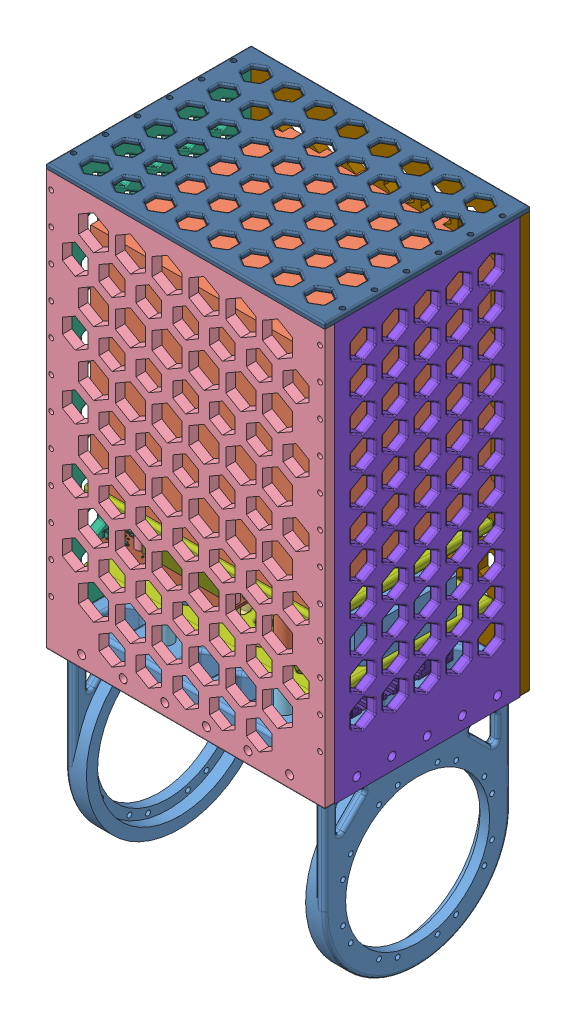
SolidWorks assembly upperbody, configuration 默认. Lengths in mm.
Overall size (174 383 128).
497 component instances, 113 part files, 71 mates.
Components (placement in the parent):
- crotch-1: crotch [默认] at (4.5084 -17.0112 162) size (162 138.05 116)
- battery-1: battery [默认] at (3.2915 206.5588 214.1011) x (-1 0 0) z (0 -1 0) size (140 115 140)
- imu-1: imu [默认] at (5.7743 27.9888 133.0371) x (0 0 -1) z (0 1 0) size (79.76 40 69.46)
- front-1: front [默认] at (4.5084 194.9888 220) size (174 260 6)
- M8螺柱-1: M8螺柱 [默认] at (42.5084 62.9888 122) size (10 25 10)
- M8螺柱-2: M8螺柱 [默认] at (42.5084 62.9888 202) x (0.721666 0 -0.692241) z (0.692241 0 0.721666) size (10 25 10)
- M8螺柱-3: M8螺柱 [默认] at (-32.4916 62.9888 122) x (0.928948 0 -0.370211) z (0.370211 0 0.928948) size (10 25 10)
- M8螺柱-4: M8螺柱 [默认] at (-32.4916 62.9888 202) x (0.697956 0 -0.71614) z (0.71614 0 0.697956) size (10 25 10)
- left-1: left [默认] at (-82.4916 204.9888 162) x (0 0 -1) z (1 0 0) size (116 260 6)
- ctrlbox-2: ctrlbox [默认] at (5.0084 87.9888 162) size (148 6 110)
- right-1: right [默认] at (91.5084 204.9888 162) x (0 0 1) z (-1 0 0) size (116 260 6)
- back-2: back [默认] at (4.5084 194.9888 98) size (174 260 6)
- top-1: top [默认] at (4.5084 304.9888 162) size (174 3 128)
- jetsonnano-1: jetsonnano [默认] at (-39.9804 116.3688 223.5192) x (0 0 1) z (0 1 0) size (100.18 80.53 31.78)
  - 675_13541_batuu_dev_kit_top_ass_asm.stp-1: 675_13541_batuu_dev_kit_top_ass_asm.stp [Default] at (-107.5192 -7.5112 -12.38) size (100.18 80.53 31.78)
    - 642-13541_BATUU_SYS_BOM_ASM.stp-1: 642-13541_BATUU_SYS_BOM_ASM.stp [Default] at origin size (100.18 80.53 21.55)
      - 600-13542-BASE-A02_ASM.stp-1: 600-13542-BASE-A02_ASM.stp [Default] at origin size (100.18 80.53 21.55)
        - 600-13542-BASE-A02.stp-1: 600-13542-BASE-A02.stp [Default] at origin size (100 79 1.57)
        - 064-0473-000_1.stp-1: 064-0473-000_1.stp [Default] at (2.055 -14.41 1.57) size (11.16 8.51 5.94)
        - LOGO_SILK_180_I560.stp-1: LOGO_SILK_180_I560.stp [Default] at (2.088 17.507 0) x (0 1 0) z (0 0 -1) size (14.3 1.27 0.05)
        - LOGO_SILK_POSTAL_ADDRESS.stp-1: LOGO_SILK_POSTAL_ADDRESS.stp [Default] at (3.985 7.597 0) x (0 1 0) z (0 0 -1) size (18.11 2.17 0.05)
        - LS_ICES_I0925X0040_CLASS_B.stp-1: LS_ICES_I0925X0040_CLASS_B.stp [Default] at (0.822 15.645 0) x (0 1 0) z (0 0 -1) size (17.94 1.42 0.03)
        - LOGO_SILK_P3542.stp-1: LOGO_SILK_P3542.stp [Default] at (-1.446 36.987 0) x (0 1 0) z (0 0 -1) size (6.18 1.16 0.01)
        - LOGO_SILK_ROHS_I0300X0153.stp-1: LOGO_SILK_ROHS_I0300X0153.stp [Default] at (0.509 33.093 0) x (0 1 0) z (0 0 -1) size (7.55 3.9 0.05)
        - LOGO_SILK_NVIDIA_I0400X0240.stp-1: LOGO_SILK_NVIDIA_I0400X0240.stp [Default] at (10.037 11.31 0) x (0 1 0) z (0 0 -1) size (7.63 5.72 0.1)
        - 115-1921-000_3.stp-1: 115-1921-000_3.stp [Default] at (71 38 1.57) x (0 -1 0) z (0 0 1) size (5 4 1.01)
        - 115-1921-000_3.stp-2: 115-1921-000_3.stp [Default] at (71 46.5 1.57) x (0 -1 0) z (0 0 1) size (5 4 1.01)
        - 115-1921-000_3.stp-3: 115-1921-000_3.stp [Default] at (71 29.5 1.57) x (0 -1 0) z (0 0 1) size (5 4 1.01)
        - LS_CTUVUS_0500X0500_SIMPLE.stp-1: LS_CTUVUS_0500X0500_SIMPLE.stp [Default] at (49.36 31.942 0) x (-1 0 0) z (0 0 -1) size (5.04 5.01 0.05)
        - LOGO_SILK_UKRAINE_0500X0500.stp-1: LOGO_SILK_UKRAINE_0500X0500.stp [Default] at (41 32.494 0) x (-1 0 0) z (0 0 -1) size (4.37 5.01 0.05)
        - LOGO_SILK_SAA_1206X0540.stp-1: LOGO_SILK_SAA_1206X0540.stp [Default] at (44.276 41.966 0) x (-1 0 0) z (0 0 -1) size (12.08 8.03 0.06)
        - 064-0476-000_1.stp-1: 064-0476-000_1.stp [Default] at (55.6 -9.269 1.57) size (14.86 17.99 18.47)
        - 064-0472-000_1.stp-1: 064-0472-000_1.stp [Default] at (88 -14.3 1.57) size (8.8 6.34 3.46)
        - 0402_SHUNT_NO.stp-1: 0402_SHUNT_NO.stp [Default] at (57.444 37.6 1.57) size (1.51 0.51 0.03)
        - 0402_SHUNT_NO.stp-2: 0402_SHUNT_NO.stp [Default] at (55.15 36.025 1.57) x (0 1 0) z (0 0 1) size (1.51 0.51 0.03)
        - 0402_SHUNT_NO.stp-3: 0402_SHUNT_NO.stp [Default] at (55.15 33.762 1.57) x (0 -1 0) z (0 0 1) size (1.51 0.51 0.03)
        - 0402_SHORT.stp-1: 0402_SHORT.stp [Default] at (57.6 38.53 1.57) size (1.51 0.51 1)
        - 0402_SHORT.stp-2: 0402_SHORT.stp [Default] at (53.708 35.675 1.57) x (-1 0 0) z (0 0 1) size (1.51 0.51 1)
        - 0402_SHORT.stp-3: 0402_SHORT.stp [Default] at (53.708 34.112 1.57) x (-1 0 0) z (0 0 1) size (1.51 0.51 1)
        - 0402_SHORT.stp-4: 0402_SHORT.stp [Default] at (60.9 37.1 1.57) x (0 -1 0) z (0 0 1) size (1.51 0.51 1)
        - 064-0474-000_1.stp-1: 064-0474-000_1.stp [Default] at (38.6 -9.759 1.57) size (14.81 17.11 9.91)
        - 085-0347-000_1.stp-1: 085-0347-000_1.stp [Default] at (31.173 31.804 1.57) x (0 -1 0) z (0 0 1) size (3.6 2.9 0.81)
        - 115-2844-000_1.stp-1: 115-2844-000_1.stp [Default] at (39.89 33.254 1.57) x (0 1 0) z (0 0 1) size (5.01 7.06 1.76)
        - 074-0259-000_1.stp-1: 074-0259-000_1.stp [Default] at (19.751 -12.06 1.57) x (0 1 0) z (0 0 1) size (13.02 16.16 8.1)
        - 106-0078-000_1.stp-1: 106-0078-000_1.stp [Default] at (4.864 -6.11 1.57) size (6.08 4.44 1.61)
        - LOGO_SILK_EAC_050X050.stp-1: LOGO_SILK_EAC_050X050.stp [Default] at (28.157 35.506 0) x (-1 0 0) z (0 0 -1) size (5 5 0.05)
        - LOGO_LABEL_PPID_0180X0050.stp-1: LOGO_LABEL_PPID_0180X0050.stp [Default] at (49.45 19.35 0) x (-1 0 0) z (0 0 -1) size (18 5 0.15)
        - 074-0221-000_3.stp-1: 074-0221-000_3.stp [Default] at (86 29 1.57) x (0 1 0) z (0 0 1) size (51.01 5.29 12.01)
        - 080-1656-000_3.stp-1: 080-1656-000_3.stp [Default] at (44 16.6 1.57) x (-1 0 0) z (0 0 1) size (77.5 26.11 9.91)
        - 080-1669-000_2.stp-1: 080-1669-000_2.stp [Default] at (0.2 29 1.57) x (0 -1 0) z (0 0 1) size (22.61 5.4 8.01)
        - 064-0400-000_1.stp-1: 064-0400-000_1.stp [Default] at (67.5 7.785 1.57) size (10.42 6.06 13.91)
        - 220-0146-000_2.stp-1: 220-0146-000_2.stp [Default] at (59.96 55.2 0) x (-1 0 0) z (0 0 -1) size (19.53 12.33 3.44)
        - 074-0239-000_1.stp-1: 074-0239-000_1.stp [Default] at (31.71 54.5 1.57) x (-1 0 0) z (0 0 1) size (30.59 10.8 5.76)
        - 0603_H100.stp-1: 0603_H100.stp [Default] at (34.617 32.966 1.57) x (0 1 0) z (0 0 1) size (1.81 1.01 1.01)
        - 0603_H100.stp-2: 0603_H100.stp [Default] at (33.893 7.175 1.57) x (-1 0 0) z (0 0 1) size (1.81 1.01 1.01)
        - 0603_H100.stp-3: 0603_H100.stp [Default] at (20.2 35 1.57) x (-1 0 0) z (0 0 1) size (1.81 1.01 1.01)
        - 0603_H100.stp-4: 0603_H100.stp [Default] at (20.2 33.55 1.57) x (-1 0 0) z (0 0 1) size (1.81 1.01 1.01)
        - 0603_H100.stp-5: 0603_H100.stp [Default] at (13.895 41.85 1.57) x (-1 0 0) z (0 0 1) size (1.81 1.01 1.01)
        - 0603_H100.stp-6: 0603_H100.stp [Default] at (7.3 3.117 1.57) size (1.81 1.01 1.01)
        - 0603_H100.stp-7: 0603_H100.stp [Default] at (11.03 6.374 1.57) x (0 1 0) z (0 0 1) size (1.81 1.01 1.01)
        - 0603_H060.stp-1: 0603_H060.stp [Default] at (63.195 1.13 1.57) size (1.81 1.02 0.61)
        - 0603_H060.stp-2: 0603_H060.stp [Default] at (82.541 -6.821 1.57) x (-1 0 0) z (0 0 1) size (1.81 1.02 0.61)
        - 0603_H060.stp-3: 0603_H060.stp [Default] at (82.541 -9.047 1.57) x (-1 0 0) z (0 0 1) size (1.81 1.02 0.61)
        - FID_40_80SM.stp-1: FID_40_80SM.stp [Default] at (80.7 59.5 1.57) size (2.29 2.29 0.05)
        - FID_40_80SM.stp-2: FID_40_80SM.stp [Default] at (7.943 54.544 1.57) size (2.29 2.29 0.05)
        - FID_40_80SM.stp-3: FID_40_80SM.stp [Default] at (93.132 -0.325 1.57) size (2.29 2.29 0.05)
        - FID_40_80SM.stp-4: FID_40_80SM.stp [Default] at (9.9 22.4 0) x (-1 0 0) z (0 0 -1) size (2.29 2.29 0.05)
        - FID_40_80SM.stp-5: FID_40_80SM.stp [Default] at (80.7 59.5 0) x (-1 0 0) z (0 0 -1) size (2.29 2.29 0.05)
        - FID_40_80SM.stp-6: FID_40_80SM.stp [Default] at (3.95 -6.475 0) x (-1 0 0) z (0 0 -1) size (2.29 2.29 0.05)
        - LOGO_SILK_ROHS_D050_CHINA.stp-1: LOGO_SILK_ROHS_D050_CHINA.stp [Default] at (35.305 32.341 0) x (-1 0 0) z (0 0 -1) size (5.62 4.99 0.05)
        - LOGO_SILK_WEEE_0485X0683.stp-1: LOGO_SILK_WEEE_0485X0683.stp [Default] at (28.183 29 0) x (-1 0 0) z (0 0 -1) size (4.85 6.82 0.05)
        - LOGO_SILK_VCCI_I0300X0225.stp-1: LOGO_SILK_VCCI_I0300X0225.stp [Default] at (55.897 33.25 0) x (-1 0 0) z (0 0 -1) size (8.32 6.14 0.05)
        - LOGO_SILK_RCM_040X030.stp-1: LOGO_SILK_RCM_040X030.stp [Default] at (57.832 27.06 0) x (-1 0 0) z (0 0 -1) size (4.05 3 0.05)
        - LOGO_SILK_BSMI_I0138H.stp-1: LOGO_SILK_BSMI_I0138H.stp [Default] at (52.892 27.23 0) x (-1 0 0) z (0 0 -1) size (8.8 3.76 0.05)
        - LOGO_SILK_HF_I0185X0120.stp-1: LOGO_SILK_HF_I0185X0120.stp [Default] at (37.6 25.2 0) x (-1 0 0) z (0 0 -1) size (4.83 3.17 0.07)
        - 090-0243-000_1.stp-1: 090-0243-000_1.stp [Default] at (88.606 -9.875 1.57) size (1.41 0.71 0.46)
        - 090-0243-000_1.stp-2: 090-0243-000_1.stp [Default] at (86.685 -9.875 1.57) x (-1 0 0) z (0 0 1) size (1.41 0.71 0.46)
        - 090-0243-000_1.stp-3: 090-0243-000_1.stp [Default] at (43.22 0.665 1.57) size (1.41 0.71 0.46)
        - 090-0243-000_1.stp-4: 090-0243-000_1.stp [Default] at (41.15 0.665 1.57) x (-1 0 0) z (0 0 1) size (1.41 0.71 0.46)
        - 090-0243-000_1.stp-5: 090-0243-000_1.stp [Default] at (11.85 27.85 1.57) size (1.41 0.71 0.46)
        - 090-0243-000_1.stp-6: 090-0243-000_1.stp [Default] at (12.358 6.374 1.57) x (0 1 0) z (0 0 1) size (1.41 0.71 0.46)
        - 090-0243-000_1.stp-7: 090-0243-000_1.stp [Default] at (19.35 -1.5 1.57) size (1.41 0.71 0.46)
        - 090-0243-000_1.stp-8: 090-0243-000_1.stp [Default] at (17.358 -1.5 1.57) size (1.41 0.71 0.46)
        - 090-0243-000_1.stp-9: 090-0243-000_1.stp [Default] at (15.308 -1.5 1.57) x (-1 0 0) z (0 0 1) size (1.41 0.71 0.46)
        - 090-0243-000_1.stp-10: 090-0243-000_1.stp [Default] at (13.064 -4.054 1.57) x (-1 0 0) z (0 0 1) size (1.41 0.71 0.46)
        - 090-0243-000_1.stp-11: 090-0243-000_1.stp [Default] at (3.491 18.432 1.57) x (0 -1 0) z (0 0 1) size (1.41 0.71 0.46)
        - 090-0243-000_1.stp-12: 090-0243-000_1.stp [Default] at (5.016 18.432 1.57) x (0 -1 0) z (0 0 1) size (1.41 0.71 0.46)
        - 090-0243-000_1.stp-13: 090-0243-000_1.stp [Default] at (11.85 23.6 1.57) size (1.41 0.71 0.46)
        - 090-0243-000_1.stp-14: 090-0243-000_1.stp [Default] at (11.85 25.25 1.57) size (1.41 0.71 0.46)
        - 090-0243-000_1.stp-15: 090-0243-000_1.stp [Default] at (11.85 26.5 1.57) size (1.41 0.71 0.46)
        - 091-0023-000_1.stp-1: 091-0023-000_1.stp [Default] at (17.098 5.642 1.57) size (2.21 2.51 1.11)
        - 115-2747-000_1.stp-1: 115-2747-000_1.stp [Default] at (11.957 32.276 1.57) x (0 1 0) z (0 0 1) size (2.21 2.88 1.11)
        - 115-0742-000_2.stp-1: 115-0742-000_2.stp [Default] at (5.725 44.6 1.57) size (2.21 2.88 1.11)
        - 115-1821-000_1.stp-1: 115-1821-000_1.stp [Default] at (12.1 48.825 1.57) x (0 -1 0) z (0 0 1) size (2.21 2.88 1.11)
        - 115-1821-000_1.stp-2: 115-1821-000_1.stp [Default] at (8.55 44.6 1.57) x (-1 0 0) z (0 0 1) size (2.21 2.88 1.11)
        - 115-0138-000_1.stp-1: 115-0138-000_1.stp [Default] at (59.536 5.825 1.57) x (-1 0 0) z (0 0 1) size (2.21 2.88 1.11)
        - 115-0742-000_2.stp-2: 115-0742-000_2.stp [Default] at (11.3 44.6 1.57) x (-1 0 0) z (0 0 1) size (2.21 2.88 1.11)
        - 315-1048-000_1.stp-1: 315-1048-000_1.stp [Default] at (7.151 6.724 1.57) x (0 1 0) z (0 0 1) size (3.11 3.58 1.46)
        - 315-1014-000_1.stp-1: 315-1014-000_1.stp [Default] at (36.977 7.376 1.57) size (3.11 3.58 1.46)
        - 315-0620-000_1.stp-1: 315-0620-000_1.stp [Default] at (53.589 41.71 1.57) x (0 -1 0) z (0 0 1) size (3.11 3.58 1.11)
        - LOGO_SILK_CE_I0175X0160.stp-1: LOGO_SILK_CE_I0175X0160.stp [Default] at (41.179 26.706 0) x (-1 0 0) z (0 0 -1) size (4.55 3.29 0.05)
        - 090-0231-000_1.stp-1: 090-0231-000_1.stp [Default] at (56.393 1.13 1.57) x (-1 0 0) z (0 0 1) size (2.61 1.55 0.56)
        - 090-0231-000_1.stp-2: 090-0231-000_1.stp [Default] at (25.625 -1.95 1.57) x (-1 0 0) z (0 0 1) size (2.61 1.55 0.56)
        - 090-0231-000_1.stp-3: 090-0231-000_1.stp [Default] at (21.95 -1.95 1.57) size (2.61 1.55 0.56)
        - 090-0231-000_1.stp-4: 090-0231-000_1.stp [Default] at (38.6 0.417 1.57) size (2.61 1.55 0.56)
        - 0402_H040.stp-1: 0402_H040.stp [Default] at (61.419 6.962 1.57) x (0 1 0) z (0 0 1) size (1.2 0.61 0.41)
        - 0402_H060.stp-1: 0402_H060.stp [Default] at (3.646 48.98 1.57) x (0 -1 0) z (0 0 1) size (1.11 0.61 0.61)
        - 0402_H060.stp-2: 0402_H060.stp [Default] at (82.141 -12.349 1.57) x (-1 0 0) z (0 0 1) size (1.11 0.61 0.61)
        - 0402_H060.stp-3: 0402_H060.stp [Default] at (85.011 -10.767 1.57) x (-1 0 0) z (0 0 1) size (1.11 0.61 0.61)
        - 0402_H040.stp-2: 0402_H040.stp [Default] at (57.017 6.2 1.57) x (0 1 0) z (0 0 1) size (1.2 0.61 0.41)
        - 0402_H060.stp-4: 0402_H060.stp [Default] at (50.674 42.15 1.57) x (0 -1 0) z (0 0 1) size (1.11 0.61 0.61)
        - 0402_H060.stp-5: 0402_H060.stp [Default] at (56.489 42.038 1.57) x (0 -1 0) z (0 0 1) size (1.11 0.61 0.61)
        - 0402_H060.stp-6: 0402_H060.stp [Default] at (9.475 49.55 1.57) x (0 1 0) z (0 0 1) size (1.11 0.61 0.61)
        - 0402_H040.stp-3: 0402_H040.stp [Default] at (35.099 35.617 1.57) size (1.2 0.61 0.41)
        - 0402_H040.stp-4: 0402_H040.stp [Default] at (37.596 37.35 1.57) x (-1 0 0) z (0 0 1) size (1.2 0.61 0.41)
        - 0402_H040.stp-5: 0402_H040.stp [Default] at (85.653 -8.168 1.57) x (0 1 0) z (0 0 1) size (1.2 0.61 0.41)
        - 0402_H060.stp-7: 0402_H060.stp [Default] at (33.493 30.304 1.57) x (0 1 0) z (0 0 1) size (1.11 0.61 0.61)
        - 0402_H060.stp-8: 0402_H060.stp [Default] at (33.493 32.251 1.57) x (0 1 0) z (0 0 1) size (1.11 0.61 0.61)
        - 0402_H060.stp-9: 0402_H060.stp [Default] at (35.099 34.667 1.57) x (-1 0 0) z (0 0 1) size (1.11 0.61 0.61)
        - 0402_H060.stp-10: 0402_H060.stp [Default] at (33.45 36.567 1.57) x (-1 0 0) z (0 0 1) size (1.11 0.61 0.61)
        - 0402_H060.stp-11: 0402_H060.stp [Default] at (33.45 35.617 1.57) x (-1 0 0) z (0 0 1) size (1.11 0.61 0.61)
        - 0402_H040.stp-6: 0402_H040.stp [Default] at (14.693 -3.538 1.57) x (0 -1 0) z (0 0 1) size (1.2 0.61 0.41)
        - 0402_H060.stp-12: 0402_H060.stp [Default] at (50.945 26.269 1.57) size (1.11 0.61 0.61)
        - 0402_H060.stp-13: 0402_H060.stp [Default] at (53.281 0.53 1.57) size (1.11 0.61 0.61)
        - 0402_H060.stp-14: 0402_H060.stp [Default] at (30.208 -2.121 1.57) x (-1 0 0) z (0 0 1) size (1.11 0.61 0.61)
        - 0402_H040.stp-7: 0402_H040.stp [Default] at (5.44 41.7 1.57) x (-1 0 0) z (0 0 1) size (1.2 0.61 0.41)
        - 0402_H060.stp-15: 0402_H060.stp [Default] at (21.109 6.878 1.57) x (0 -1 0) z (0 0 1) size (1.11 0.61 0.61)
        - 0402_H040.stp-8: 0402_H040.stp [Default] at (12.1 46.85 1.57) size (1.2 0.61 0.41)
        - 0402_H040.stp-9: 0402_H040.stp [Default] at (89.1 -4.75 1.57) x (-1 0 0) z (0 0 1) size (1.2 0.61 0.41)
        - 0402_H040.stp-10: 0402_H040.stp [Default] at (73.778 10.336 1.57) x (-1 0 0) z (0 0 1) size (1.2 0.61 0.41)
        - 0402_H040.stp-11: 0402_H040.stp [Default] at (16.95 -0.35 1.57) x (-1 0 0) z (0 0 1) size (1.2 0.61 0.41)
        - 0402_H040.stp-12: 0402_H040.stp [Default] at (15.333 -0.35 1.57) size (1.2 0.61 0.41)
        - 0402_H040.stp-13: 0402_H040.stp [Default] at (18.957 4.734 1.57) x (0 1 0) z (0 0 1) size (1.2 0.61 0.41)
        - 0402_H040.stp-14: 0402_H040.stp [Default] at (14.912 7.235 1.57) x (-1 0 0) z (0 0 1) size (1.2 0.61 0.41)
        - 0402_H040.stp-15: 0402_H040.stp [Default] at (31.504 6.574 1.57) x (-1 0 0) z (0 0 1) size (1.2 0.61 0.41)
        - 0402_H040.stp-16: 0402_H040.stp [Default] at (29.859 6.574 1.57) size (1.2 0.61 0.41)
        - 0402_H060.stp-16: 0402_H060.stp [Default] at (38.505 2.843 1.57) x (0 -1 0) z (0 0 1) size (1.11 0.61 0.61)
        - 0402_H060.stp-17: 0402_H060.stp [Default] at (34.05 8.75 1.57) x (-1 0 0) z (0 0 1) size (1.11 0.61 0.61)
        - 0402_H060.stp-18: 0402_H060.stp [Default] at (37.594 2.843 1.57) x (0 -1 0) z (0 0 1) size (1.11 0.61 0.61)
        - 0402_H040.stp-17: 0402_H040.stp [Default] at (44.5 9.25 1.57) size (1.2 0.61 0.41)
        - 0402_H040.stp-18: 0402_H040.stp [Default] at (6.98 47.3 1.57) size (1.2 0.61 0.41)
        - 0402_H040.stp-19: 0402_H040.stp [Default] at (82.141 -11.445 1.57) x (-1 0 0) z (0 0 1) size (1.2 0.61 0.41)
        - 0402_H040.stp-20: 0402_H040.stp [Default] at (63.62 -11.35 1.57) x (0 -1 0) z (0 0 1) size (1.2 0.61 0.41)
        - 0402_H060.stp-19: 0402_H060.stp [Default] at (39.409 2.843 1.57) x (0 -1 0) z (0 0 1) size (1.11 0.61 0.61)
        - 0402_H060.stp-20: 0402_H060.stp [Default] at (40.35 2.843 1.57) x (0 -1 0) z (0 0 1) size (1.11 0.61 0.61)
        - 0402_H060.stp-21: 0402_H060.stp [Default] at (4.425 -9.55 1.57) size (1.11 0.61 0.61)
        - 0402_H060.stp-22: 0402_H060.stp [Default] at (26.7 47 1.57) size (1.11 0.61 0.61)
        - 0402_H070.stp-1: 0402_H070.stp [Default] at (20.2 36.2 1.57) x (-1 0 0) z (0 0 1) size (1.11 0.61 0.71)
        - 0402_H060.stp-23: 0402_H060.stp [Default] at (5.44 40.55 1.57) size (1.11 0.61 0.61)
        - 0402_H060.stp-24: 0402_H060.stp [Default] at (57.017 7.825 1.57) x (0 1 0) z (0 0 1) size (1.11 0.61 0.61)
        - 0402_H060.stp-25: 0402_H060.stp [Default] at (73.65 4 1.57) size (1.11 0.61 0.61)
        - 0402_H060.stp-26: 0402_H060.stp [Default] at (82.141 -10.442 1.57) size (1.11 0.61 0.61)
        - 0402_H060.stp-27: 0402_H060.stp [Default] at (63.37 3.231 1.57) size (1.11 0.61 0.61)
        - 0402_H060.stp-28: 0402_H060.stp [Default] at (6.652 4.356 1.57) size (1.11 0.61 0.61)
        - 0402_H060.stp-29: 0402_H060.stp [Default] at (24.377 6.917 1.57) x (0 -1 0) z (0 0 1) size (1.11 0.61 0.61)
        - 0402_H060.stp-30: 0402_H060.stp [Default] at (27.693 6.896 1.57) x (0 -1 0) z (0 0 1) size (1.11 0.61 0.61)
        - 0402_H060.stp-31: 0402_H060.stp [Default] at (30.18 7.846 1.57) x (0 -1 0) z (0 0 1) size (1.11 0.61 0.61)
        - 0402_H060.stp-32: 0402_H060.stp [Default] at (22.059 6.878 1.57) x (0 -1 0) z (0 0 1) size (1.11 0.61 0.61)
        - 0402_H060.stp-33: 0402_H060.stp [Default] at (25.377 6.917 1.57) x (0 -1 0) z (0 0 1) size (1.11 0.61 0.61)
        - 0402_H060.stp-34: 0402_H060.stp [Default] at (28.602 6.896 1.57) x (0 -1 0) z (0 0 1) size (1.11 0.61 0.61)
        - 0402_H060.stp-35: 0402_H060.stp [Default] at (31.154 7.846 1.57) x (0 -1 0) z (0 0 1) size (1.11 0.61 0.61)
        - 0402_H060.stp-36: 0402_H060.stp [Default] at (15.954 -4.338 1.57) size (1.11 0.61 0.61)
        - 0402_H060.stp-37: 0402_H060.stp [Default] at (13.93 5.406 1.57) x (-1 0 0) z (0 0 1) size (1.11 0.61 0.61)
        - 0402_H060.stp-38: 0402_H060.stp [Default] at (15.95 -2.95 1.57) x (-1 0 0) z (0 0 1) size (1.11 0.61 0.61)
        - 0402_H060.stp-39: 0402_H060.stp [Default] at (19.2 -2.95 1.57) size (1.11 0.61 0.61)
        - 0402_H060.stp-40: 0402_H060.stp [Default] at (17.551 -2.95 1.57) size (1.11 0.61 0.61)
        - 0402_H060.stp-41: 0402_H060.stp [Default] at (13.064 -2.95 1.57) x (-1 0 0) z (0 0 1) size (1.11 0.61 0.61)
        - 0402_H060.stp-42: 0402_H060.stp [Default] at (2.85 37.55 1.57) x (0 1 0) z (0 0 1) size (1.11 0.61 0.61)
        - 0402_H060.stp-43: 0402_H060.stp [Default] at (68.15 40.157 1.57) x (0 1 0) z (0 0 1) size (1.11 0.61 0.61)
        - 0402_H060.stp-44: 0402_H060.stp [Default] at (73.85 40.157 1.57) x (0 1 0) z (0 0 1) size (1.11 0.61 0.61)
        - 0402_H060.stp-45: 0402_H060.stp [Default] at (90.95 6.1 1.57) size (1.11 0.61 0.61)
        - 0402_H060.stp-46: 0402_H060.stp [Default] at (68.167 49.132 1.57) x (0 1 0) z (0 0 1) size (1.11 0.61 0.61)
        - 0402_H060.stp-47: 0402_H060.stp [Default] at (59.769 3.59 1.57) x (-1 0 0) z (0 0 1) size (1.11 0.61 0.61)
        - 0402_H060.stp-48: 0402_H060.stp [Default] at (73.85 48.646 1.57) x (0 1 0) z (0 0 1) size (1.11 0.61 0.61)
        - 0402_H060.stp-49: 0402_H060.stp [Default] at (68.15 31.652 1.57) x (0 1 0) z (0 0 1) size (1.11 0.61 0.61)
        - 0402_H060.stp-50: 0402_H060.stp [Default] at (73.85 31.66 1.57) x (0 1 0) z (0 0 1) size (1.11 0.61 0.61)
        - 0402_H060.stp-51: 0402_H060.stp [Default] at (39.15 45.85 1.57) x (-1 0 0) z (0 0 1) size (1.11 0.61 0.61)
        - 0402_H060.stp-52: 0402_H060.stp [Default] at (39.15 46.878 1.57) x (-1 0 0) z (0 0 1) size (1.11 0.61 0.61)
        - 0402_H060.stp-53: 0402_H060.stp [Default] at (73.778 8.083 1.57) x (0 -1 0) z (0 0 1) size (1.11 0.61 0.61)
        - 0402_H060.stp-54: 0402_H060.stp [Default] at (27.5 49.75 1.57) x (-1 0 0) z (0 0 1) size (1.11 0.61 0.61)
        - 0402_H060.stp-55: 0402_H060.stp [Default] at (59.5 37.1 1.57) x (-1 0 0) z (0 0 1) size (1.11 0.61 0.61)
        - 0402_H040.stp-21: 0402_H040.stp [Default] at (14.621 0.778 1.57) x (-1 0 0) z (0 0 1) size (1.2 0.61 0.41)
        - 0402_H040.stp-22: 0402_H040.stp [Default] at (14.887 6.314 1.57) size (1.2 0.61 0.41)
        - 0402_H040.stp-23: 0402_H040.stp [Default] at (13.555 7.126 1.57) x (0 -1 0) z (0 0 1) size (1.2 0.61 0.41)
        - 0402_H040.stp-24: 0402_H040.stp [Default] at (12.661 0.478 1.57) x (0 1 0) z (0 0 1) size (1.2 0.61 0.41)
        - 0402_H040.stp-25: 0402_H040.stp [Default] at (53.55 23.2 1.57) x (0 1 0) z (0 0 1) size (1.2 0.61 0.41)
        - 0402_H040.stp-26: 0402_H040.stp [Default] at (57.842 9.9 1.57) x (0 1 0) z (0 0 1) size (1.2 0.61 0.41)
        - 0402_H040.stp-27: 0402_H040.stp [Default] at (58.75 9.9 1.57) x (0 1 0) z (0 0 1) size (1.2 0.61 0.41)
        - 0402_H040.stp-28: 0402_H040.stp [Default] at (60.45 32.794 1.57) x (0 1 0) z (0 0 1) size (1.2 0.61 0.41)
        - 0402_H040.stp-29: 0402_H040.stp [Default] at (61.787 35.7 1.57) x (0 -1 0) z (0 0 1) size (1.2 0.61 0.41)
        - 0402_H040.stp-30: 0402_H040.stp [Default] at (60.15 9.9 1.57) x (0 1 0) z (0 0 1) size (1.2 0.61 0.41)
        - 0402_H040.stp-31: 0402_H040.stp [Default] at (3.646 43.6 1.57) x (0 1 0) z (0 0 1) size (1.2 0.61 0.41)
        - 0402_H040.stp-32: 0402_H040.stp [Default] at (61.075 9.9 1.57) x (0 1 0) z (0 0 1) size (1.2 0.61 0.41)
        - 0402_H040.stp-33: 0402_H040.stp [Default] at (13 36.398 1.57) x (0 -1 0) z (0 0 1) size (1.2 0.61 0.41)
        - 0402_H040.stp-34: 0402_H040.stp [Default] at (11.693 36.398 1.57) x (0 -1 0) z (0 0 1) size (1.2 0.61 0.41)
        - 0402_H040.stp-35: 0402_H040.stp [Default] at (-1.925 -7.511 1.57) x (-1 0 0) z (0 0 1) size (1.2 0.61 0.41)
        - 0402_H040.stp-36: 0402_H040.stp [Default] at (-1.925 -6.588 1.57) x (-1 0 0) z (0 0 1) size (1.2 0.61 0.41)
        - 0402_H040.stp-37: 0402_H040.stp [Default] at (10.28 1.69 1.57) x (0 1 0) z (0 0 1) size (1.2 0.61 0.41)
        - 0402_H040.stp-38: 0402_H040.stp [Default] at (11.49 -3.788 1.57) x (0 -1 0) z (0 0 1) size (1.2 0.61 0.41)
        - 0402_H040.stp-39: 0402_H040.stp [Default] at (35.418 10.679 1.57) x (0 1 0) z (0 0 1) size (1.2 0.61 0.41)
        - 0402_H040.stp-40: 0402_H040.stp [Default] at (41.66 2.685 1.57) x (0 -1 0) z (0 0 1) size (1.2 0.61 0.41)
        - 0402_H040.stp-41: 0402_H040.stp [Default] at (42.61 2.685 1.57) x (0 -1 0) z (0 0 1) size (1.2 0.61 0.41)
        - 0402_H040.stp-42: 0402_H040.stp [Default] at (50.15 1.275 1.57) size (1.2 0.61 0.41)
        - 0402_H040.stp-43: 0402_H040.stp [Default] at (50.15 2.225 1.57) size (1.2 0.61 0.41)
        - 0402_H040.stp-44: 0402_H040.stp [Default] at (50.173 3.305 1.57) size (1.2 0.61 0.41)
        - 0402_H040.stp-45: 0402_H040.stp [Default] at (50.173 4.255 1.57) size (1.2 0.61 0.41)
        - 0402_H040.stp-46: 0402_H040.stp [Default] at (53.589 39.034 1.57) x (-1 0 0) z (0 0 1) size (1.2 0.61 0.41)
        - 0402_H040.stp-47: 0402_H040.stp [Default] at (24.4 47.25 1.57) x (0 1 0) z (0 0 1) size (1.2 0.61 0.41)
        - 0402_H040.stp-48: 0402_H040.stp [Default] at (26.7 47.9 1.57) size (1.2 0.61 0.41)
        - 0402_H040.stp-49: 0402_H040.stp [Default] at (25.9 48.85 1.57) x (-1 0 0) z (0 0 1) size (1.2 0.61 0.41)
        - 0402_H040.stp-50: 0402_H040.stp [Default] at (7.975 41.7 1.57) x (-1 0 0) z (0 0 1) size (1.2 0.61 0.41)
        - 0402_H040.stp-51: 0402_H040.stp [Default] at (14.095 40.55 1.57) size (1.2 0.61 0.41)
        - 0402_H040.stp-52: 0402_H040.stp [Default] at (61.419 5.325 1.57) x (0 1 0) z (0 0 1) size (1.2 0.61 0.41)
        - 0402_H040.stp-53: 0402_H040.stp [Default] at (11.3 42.2 1.57) x (-1 0 0) z (0 0 1) size (1.2 0.61 0.41)
        - 0402_H040.stp-54: 0402_H040.stp [Default] at (5.375 47.3 1.57) size (1.2 0.61 0.41)
        - 0402_H040.stp-55: 0402_H040.stp [Default] at (82.541 -5.697 1.57) x (-1 0 0) z (0 0 1) size (1.2 0.61 0.41)
        - 0402_H040.stp-56: 0402_H040.stp [Default] at (82.141 -7.946 1.57) x (-1 0 0) z (0 0 1) size (1.2 0.61 0.41)
        - 0402_H040.stp-57: 0402_H040.stp [Default] at (63.37 2.26 1.57) size (1.2 0.61 0.41)
        - 0402_H040.stp-58: 0402_H040.stp [Default] at (52.6 23.2 1.57) x (0 1 0) z (0 0 1) size (1.2 0.61 0.41)
        - 0402_H040.stp-59: 0402_H040.stp [Default] at (15.583 8.9 1.57) x (0 -1 0) z (0 0 1) size (1.2 0.61 0.41)
        - 0402_H040.stp-60: 0402_H040.stp [Default] at (10.426 8.65 1.57) size (1.2 0.61 0.41)
        - 0402_H040.stp-61: 0402_H040.stp [Default] at (20.747 5.624 1.57) size (1.2 0.61 0.41)
        - 0402_H040.stp-62: 0402_H040.stp [Default] at (22.405 5.624 1.57) x (-1 0 0) z (0 0 1) size (1.2 0.61 0.41)
        - 0402_H040.stp-63: 0402_H040.stp [Default] at (24.029 5.624 1.57) size (1.2 0.61 0.41)
        - 0402_H040.stp-64: 0402_H040.stp [Default] at (25.662 5.624 1.57) x (-1 0 0) z (0 0 1) size (1.2 0.61 0.41)
        - 0402_H040.stp-65: 0402_H040.stp [Default] at (27.303 5.624 1.57) size (1.2 0.61 0.41)
        - 0402_H040.stp-66: 0402_H040.stp [Default] at (28.913 5.624 1.57) x (-1 0 0) z (0 0 1) size (1.2 0.61 0.41)
        - 0402_H040.stp-67: 0402_H040.stp [Default] at (20.725 2.15 1.57) x (0 -1 0) z (0 0 1) size (1.2 0.61 0.41)
        - 0402_H040.stp-68: 0402_H040.stp [Default] at (21.675 2.15 1.57) x (0 -1 0) z (0 0 1) size (1.2 0.61 0.41)
        - 0402_H040.stp-69: 0402_H040.stp [Default] at (23.225 2.15 1.57) x (0 -1 0) z (0 0 1) size (1.2 0.61 0.41)
        - 0402_H040.stp-70: 0402_H040.stp [Default] at (24.175 2.15 1.57) x (0 -1 0) z (0 0 1) size (1.2 0.61 0.41)
        - 0402_H040.stp-71: 0402_H040.stp [Default] at (25.725 2.15 1.57) x (0 -1 0) z (0 0 1) size (1.2 0.61 0.41)
        - 0402_H040.stp-72: 0402_H040.stp [Default] at (26.675 2.15 1.57) x (0 -1 0) z (0 0 1) size (1.2 0.61 0.41)
        - 0402_H040.stp-73: 0402_H040.stp [Default] at (28.225 2.15 1.57) x (0 -1 0) z (0 0 1) size (1.2 0.61 0.41)
        - 0402_H040.stp-74: 0402_H040.stp [Default] at (29.175 2.15 1.57) x (0 -1 0) z (0 0 1) size (1.2 0.61 0.41)
        - 0402_H040.stp-75: 0402_H040.stp [Default] at (12.661 -1.2 1.57) x (0 1 0) z (0 0 1) size (1.2 0.61 0.41)
        - 0402_H040.stp-76: 0402_H040.stp [Default] at (71.114 43.15 1.57) x (-1 0 0) z (0 0 1) size (1.2 0.61 0.41)
        - 0402_H040.stp-77: 0402_H040.stp [Default] at (71.522 34.65 1.57) x (-1 0 0) z (0 0 1) size (1.2 0.61 0.41)
        - 0402_H040.stp-78: 0402_H040.stp [Default] at (57.283 28.368 1.57) x (-1 0 0) z (0 0 1) size (1.2 0.61 0.41)
        - 0402_H040.stp-79: 0402_H040.stp [Default] at (43.941 46.958 1.57) x (-1 0 0) z (0 0 1) size (1.2 0.61 0.41)
        - 0402_H040.stp-80: 0402_H040.stp [Default] at (44.719 46.023 1.57) size (1.2 0.61 0.41)
        - 0402_H040.stp-81: 0402_H040.stp [Default] at (54.672 26.901 1.57) x (0 1 0) z (0 0 1) size (1.2 0.61 0.41)
        - 0402_H040.stp-82: 0402_H040.stp [Default] at (63.1 24.2 1.57) x (0 1 0) z (0 0 1) size (1.2 0.61 0.41)
        - 0402_H040.stp-83: 0402_H040.stp [Default] at (40.75 48.3 1.57) size (1.2 0.61 0.41)
        - 0402_H040.stp-84: 0402_H040.stp [Default] at (44.5 10.25 1.57) size (1.2 0.61 0.41)
        - 0402_H040.stp-85: 0402_H040.stp [Default] at (54.5 23.2 1.57) x (0 1 0) z (0 0 1) size (1.2 0.61 0.41)
        - 0402_H040.stp-86: 0402_H040.stp [Default] at (46.176 10.25 1.57) x (-1 0 0) z (0 0 1) size (1.2 0.61 0.41)
        - 0402_H040.stp-87: 0402_H040.stp [Default] at (46.08 48.3 1.57) size (1.2 0.61 0.41)
        - LTPB071C125D045C025P.stp-1: LTPB071C125D045C025P.stp [Default] at (61.144 33.25 0) x (0 -1 0) z (0 0 -1) size (0.71 0.71 0.08)
        - LTPB071C125D045C025P.stp-2: LTPB071C125D045C025P.stp [Default] at (61.144 34.6 0) x (0 -1 0) z (0 0 -1) size (0.71 0.71 0.08)
        - 032-1441-000_1.stp-1: 032-1441-000_1.stp [Default] at (33.253 2.453 1.57) x (-1 0 0) z (0 0 1) size (6.81 6.81 12.51)
        - 032-1441-000_1.stp-2: 032-1441-000_1.stp [Default] at (78.091 7.247 1.57) x (-1 0 0) z (0 0 1) size (6.81 6.81 12.51)
        - 090-0348-000_1.stp-1: 090-0348-000_1.stp [Default] at (9.3 -9.686 1.57) x (0 -1 0) z (0 0 1) size (4.36 1.81 1.36)
        - 090-0155-000_1.stp-1: 090-0155-000_1.stp [Default] at (72.55 51.651 0) x (0 1 0) z (0 0 -1) size (4.36 1.81 1.26)
        - 0805_H150.stp-1: 0805_H150.stp [Default] at (-0.7 -8.925 1.57) x (-1 0 0) z (0 0 1) size (2.22 1.46 1.51)
        - 0805_H150.stp-2: 0805_H150.stp [Default] at (29.2 46.45 1.57) x (0 1 0) z (0 0 1) size (2.22 1.46 1.51)
        - 090-0096-000_1.stp-1: 090-0096-000_1.stp [Default] at (6.98 48.475 1.57) size (1.2 0.66 0.41)
        - 092-0073-000_1.stp-1: 092-0073-000_1.stp [Default] at (93.35 -4.75 1.57) x (-1 0 0) z (0 0 1) size (2.46 1.06 0.91)
        - 102-0037-000_1.stp-1: 102-0037-000_1.stp [Default] at (42.135 2.685 1.57) size (1.08 1.86 0.92)
        - 102-0037-000_1.stp-2: 102-0037-000_1.stp [Default] at (50.15 1.75 1.57) x (0 -1 0) z (0 0 1) size (1.08 1.86 0.92)
        - 102-0066-000_2.stp-1: 102-0066-000_2.stp [Default] at (21.2 2.15 1.57) x (-1 0 0) z (0 0 1) size (1.08 1.86 0.62)
        - 102-0066-000_2.stp-2: 102-0066-000_2.stp [Default] at (23.7 2.15 1.57) x (-1 0 0) z (0 0 1) size (1.08 1.86 0.62)
        - 102-0066-000_2.stp-3: 102-0066-000_2.stp [Default] at (26.2 2.15 1.57) x (-1 0 0) z (0 0 1) size (1.08 1.86 0.62)
        - 102-0066-000_2.stp-4: 102-0066-000_2.stp [Default] at (28.7 2.15 1.57) x (-1 0 0) z (0 0 1) size (1.08 1.86 0.62)
        - 102-0037-000_1.stp-3: 102-0037-000_1.stp [Default] at (50.173 3.78 1.57) x (0 -1 0) z (0 0 1) size (1.08 1.86 0.92)
        - 131-0595-000_1.stp-1: 131-0595-000_1.stp [Default] at (24.65 39.7 1.57) x (-1 0 0) z (0 0 1) size (4.21 4.62 1.81)
        - 130-1334-000_1.stp-1: 130-1334-000_1.stp [Default] at (24.65 39.7 1.57) x (-1 0 0) z (0 0 1) size (6.5 6.31 2.11)
        - 300-0402-000_1.stp-1: 300-0402-000_1.stp [Default] at (56.787 26.503 1.57) x (0 -1 0) z (0 0 1) size (2.21 2.69 1.11)
        - 300-0402-000_1.stp-2: 300-0402-000_1.stp [Default] at (14.693 3.31 1.57) size (2.21 2.69 1.11)
        - 300-0906-000_1.stp-1: 300-0906-000_1.stp [Default] at (10.75 -0.9 1.57) size (2.21 2.69 1.11)
        - 300-0560-000_1.stp-1: 300-0560-000_1.stp [Default] at (14.095 44.6 1.57) x (-1 0 0) z (0 0 1) size (2.21 2.69 1.11)
        - 115-1566-000_1.stp-1: 115-1566-000_1.stp [Default] at (50.674 23.75 1.57) size (2.21 2.69 1.11)
        - 300-1132-000_1.stp-1: 300-1132-000_1.stp [Default] at (89.1 -7.144 1.57) x (0 1 0) z (0 0 1) size (3.11 3.2 1.17)
        - 300-1132-000_1.stp-2: 300-1132-000_1.stp [Default] at (49.309 7.122 1.57) x (-1 0 0) z (0 0 1) size (3.11 3.2 1.17)
        - 300-9001-000_1.stp-1: 300-9001-000_1.stp [Default] at (18.296 9.15 1.57) x (0 -1 0) z (0 0 1) size (3.11 3.2 1.21)
        - 300-9001-000_1.stp-2: 300-9001-000_1.stp [Default] at (17.825 2.02 1.57) x (-1 0 0) z (0 0 1) size (3.11 3.2 1.21)
        - 300-1132-000_1.stp-3: 300-1132-000_1.stp [Default] at (60.644 24.2 1.57) x (0 1 0) z (0 0 1) size (3.11 3.2 1.17)
        - 300-1132-000_1.stp-4: 300-1132-000_1.stp [Default] at (53.281 7.119 1.57) size (3.11 3.2 1.17)
        - 300-1000-000_2.stp-1: 300-1000-000_2.stp [Default] at (6.717 -1.5 1.57) x (-1 0 0) z (0 0 1) size (3.6 3.75 1.01)
        - 300-1128-000_1.stp-1: 300-1128-000_1.stp [Default] at (11.989 3.346 1.57) x (-1 0 0) z (0 0 1) size (2.21 2.8 1.11)
        - 1206_H070.stp-1: 1206_H070.stp [Default] at (4.892 -7.138 1.57) size (3.41 1.81 0.71)
        - 1206_H070.stp-2: 1206_H070.stp [Default] at (4.892 -5 1.57) size (3.41 1.81 0.71)
        - 174-0159-000_2.stp-1: 174-0159-000_2.stp [Default] at (58.5 35 1.57) x (0 -1 0) z (0 0 1) size (2 3.52 0.6)
        - 316-0758-000_1.stp-1: 316-0758-000_1.stp [Default] at (27.05 45.2 1.57) size (1.71 1.7 0.61)
        - 115-2177-000_2.stp-1: 115-2177-000_2.stp [Default] at (41.5 46.478 1.57) size (2.01 1.71 0.41)
        - 065-0743-000_1.stp-1: 065-0743-000_1.stp [Default] at (72.95 -7.46 1.57) x (-1 0 0) z (0 0 1) size (17.8 21.61 17.51)
      - 699-13448_PORG_MODULE_PCB_ASSY_ASM.stp-1: 699-13448_PORG_MODULE_PCB_ASSY_ASM.stp [Default] at (11.2 22.5 8.2662) size (69.6 45 4.71)
        - 600-13448_PORG_MODULE_PCB_ASSY_ASM.stp-1: 600-13448_PORG_MODULE_PCB_ASSY_ASM.stp [Default] at origin size (69.6 45 4.71)
          - 142-63448-1GEN_A00.stp-1: 142-63448-1GEN_A00.stp [Default] at origin size (69.6 45 4.71)
    - 682-13450_PORG_ME_THER_ASSY_ASM.stp-1: 682-13450_PORG_ME_THER_ASSY_ASM.stp [Default] at origin size (68.74 39.4 29.1)
      - PORG_HSK_ASSY_ASM.stp-1: PORG_HSK_ASSY_ASM.stp [Default] at (11.1999 22.5001 10.7662) x (1 -0.000006 0) z (0 0 1) size (58.7 39.4 17.31)
        - 110-0111-000.stp-1: 110-0111-000.stp [Default] at (0 0 1.505) size (58.7 39.4 17.31)
      - PORG_LEAF_SPRING_DRAWN.stp-1: PORG_LEAF_SPRING_DRAWN.stp [Default] at (11.2001 22.4999 7.8662) x (1 0.000006 0) z (0 0 1) size (39.83 21.3 0.8)
      - 155-0746-000.stp-1: 155-0746-000.stp [Default] at (12.2 58.5 1.57) size (5.14 4.45 6.58)
      - 155-0746-000.stp-2: 155-0746-000.stp [Default] at (75.8 58.5 1.57) size (5.14 4.45 6.58)
      - 155-0754-000.stp-1: 155-0754-000.stp [Default] at (12.2 58.5 5.7662) x (-1 0 0) z (0 0 -1) size (4.55 4.55 4.53)
      - 155-0754-000.stp-2: 155-0754-000.stp [Default] at (75.8 58.5 5.7662) x (-1 0 0) z (0 0 -1) size (4.55 4.55 4.53)
      - 155-0754-000.stp-3: 155-0754-000.stp [Default] at (12.2 58.5 3.7) size (4.55 4.55 4.53)
      - 155-0754-000.stp-4: 155-0754-000.stp [Default] at (75.8 58.5 3.7) size (4.55 4.55 4.53)
      - 155-0717-000.stp-1: 155-0717-000.stp [Default] at (18.187 28.498 11.9662) x (0 0 -1) z (0 1 0) size (6.41 4.7 4.7)
      - 155-0717-000.stp-2: 155-0717-000.stp [Default] at (18.187 43.402 11.9662) x (0 0 -1) z (0 1 0) size (6.41 4.7 4.7)
      - 155-0717-000.stp-3: 155-0717-000.stp [Default] at (51.613 43.402 11.9662) x (0 0 -1) z (0 1 0) size (6.41 4.7 4.7)
      - 155-0717-000.stp-4: 155-0717-000.stp [Default] at (51.613 28.498 11.9662) x (0 0 -1) z (0 1 0) size (6.41 4.7 4.7)
